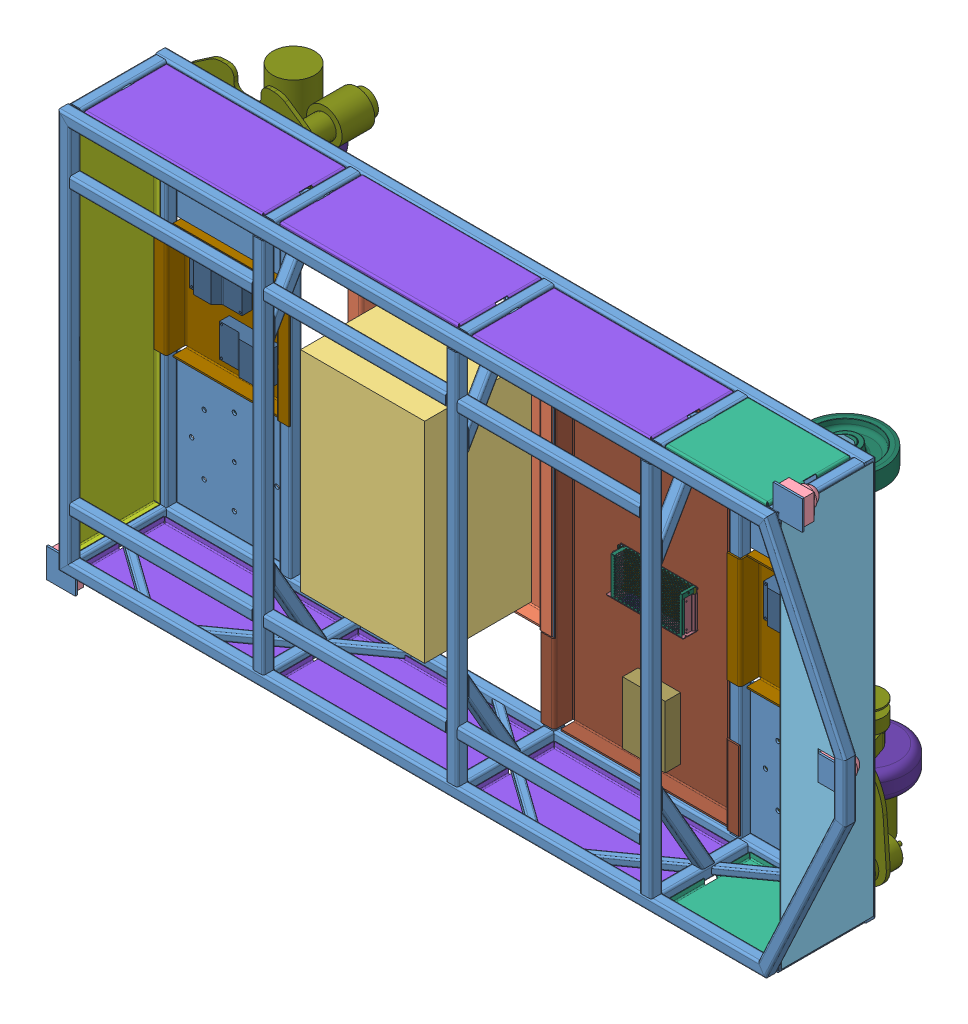
SolidWorks assembly spartaco_bot, configuration Default. Lengths in mm.
Overall size (2090 1155 574.19).
68 component instances, 36 part files, 77 mates.
Components (placement in the parent):
- 00-P-PT0151-1: 00-P-PT0151 [Default<A macchina>] at (-901.7891 -500.1516 -100.979) x (0 -1 0) z (-1 0 0) size (1155 285 2090)
- 00-P-PT0154-1: 00-P-PT0154 [Default] at (-151.7891 -0.1516 -135.979) x (1 0 0) z (0 -1 0) size (525 54 559)
- batteria-1: batteria [Default] at (-151.7891 -0.1516 -131.979) x (0 -1 0) z (-1 0 0) size (569 275 320)
- lidar-1: lidar [Default] at (940.7109 542.3484 129.021) x (0 -1 0) z (0 0 -1) size (73 65 60)
- lidar-2: lidar [Default] at (1050.7109 -0.1516 134.021) x (-1 0 0) z (0 0 -1) size (73 65 60)
- lidar-3: lidar [Default] at (-944.2891 -547.6516 129.021) x (0 1 0) z (0 0 -1) size (73 65 60)
- Parte13-1: Parte13 [Default] at (914.7109 -0.1516 -107.479) x (0 1 0) z (1 0 0) size (1015 241.5 195)
- Parte14-1: Parte14 [Default] at (750.7109 -515.1516 21.521) x (1 0 0) z (0 -1 0) size (265 215 15)
- Parte14-2: Parte14 [Default] at (745.7109 514.8484 21.521) x (-1 0 0) z (0 1 0) size (265 215 15)
- 00-P-PT0152-1: 00-P-PT0152 [Default] at (-916.7891 -2.6516 21.521) x (0 1 0) z (-1 0 0) size (965 215 15)
- 00-P-PT0153-1: 00-P-PT0153 [Default] at (-649.2891 514.8484 26.521) x (-1 0 0) z (0 1 0) size (465 215 15)
- 00-P-PT0153-2: 00-P-PT0153 [Default] at (-149.2891 514.8484 21.521) x (-1 0 0) z (0 1 0) size (465 215 15)
- 00-P-PT0153-3: 00-P-PT0153 [Default] at (350.7109 514.8484 26.521) x (-1 0 0) z (0 1 0) size (465 215 15)
- 00-P-PT0153-4: 00-P-PT0153 [Default] at (-654.2891 -515.1516 26.521) x (1 0 0) z (0 -1 0) size (465 215 15)
- 00-P-PT0153-5: 00-P-PT0153 [Default] at (-154.2891 -515.1516 26.521) x (1 0 0) z (0 -1 0) size (465 215 15)
- 00-P-PT0153-6: 00-P-PT0153 [Default] at (350.7109 -515.1516 26.521) x (1 0 0) z (0 -1 0) size (465 215 15)
- Parte17-1: Parte17 [Default] at (-1.7891 -0.1516 165.521) x (-1 0 0) z (0 1 0) size (2000 1.5 1000) (hidden)
- inverter_box-1: inverter_box [Default] at (738.2109 -0.1516 -120.7531) x (1 0 0) z (0 -1 0) size (350 54 299)
  - 00-P-PT0154-2-1: 00-P-PT0154-2 [Default] at (0 -15.2259 0) size (350 54 299)
  - minitraction_power_mockup-1: minitraction_power_mockup [Default] at (-36 -11.2259 -63) x (0 0 -1) z (0 1 0) size (85 130 40)
  - minitraction_power_mockup-2: minitraction_power_mockup [Default] at (36 -11.2259 63) x (0 0 1) z (0 1 0) size (85 130 40)
- inverter_box-2: inverter_box [Default] at (-741.7891 -0.1516 -120.7531) x (1 0 0) z (0 -1 0) size (350 54 299)
  - 00-P-PT0154-2-1: 00-P-PT0154-2 [Default] at (0 -15.2259 0) size (350 54 299)
  - minitraction_power_mockup-1: minitraction_power_mockup [Default] at (-36 -11.2259 -63) x (0 0 -1) z (0 1 0) size (85 130 40)
  - minitraction_power_mockup-2: minitraction_power_mockup [Default] at (36 -11.2259 63) x (0 0 1) z (0 1 0) size (85 130 40)
- electric_box-1: electric_box [Default] at (338.2109 -0.1516 -126.875) x (1 0 0) z (0 -1 0) size (510 54 969)
  - 00-P-PT0154-3-1: 00-P-PT0154-3 [Default] at (0 -9.104 0) size (510 54 969)
  - panda_mockup-1: panda_mockup [Default] at (0 -1.504 360.5) x (1 0 0) z (0 -1 0) size (110 160 39.6)
  - SD-100C-12-1: SD-100C-12 [Default] at (0 -3.604 71.625) size (199.09 37.75 98.27)
    - SD-100C-12.stp-1: SD-100C-12.stp [Default] at origin size (199.09 37.75 98.27)
      - SD-100-20201028.stp.stp-1: SD-100-20201028.stp.stp [Default] at origin size (199.09 37.75 98.27)
        - SD-100_STP.ASM.stp-1: SD-100_STP.ASM.stp [Default] at origin size (199.09 37.75 98.27)
          - SD-100_1_ASM.ASM.stp-1: SD-100_1_ASM.ASM.stp [Default] at origin size (199 37.75 98.27)
            - 902-D-80_ASM.ASM.stp-1: 902-D-80_ASM.ASM.stp [Default] at origin size (199 37.75 97.75)
              - 902-D-119_PRT.PRT.stp-1: 902-D-119_PRT.PRT.stp [Default] at origin size (199 37.75 97.75)
              - NUT_PRT.PRT.stp-1: NUT_PRT.PRT.stp [Default] at (-111.528 -1.5 -40.7894) x (-1 0 0) z (0 1 0) size (8 6.93 6)
            - 902-T_PRT.PRT.stp-1: 902-T_PRT.PRT.stp [Default] at (96.5 36.1 -49.375) x (-1 0 0) z (0 0 -1) size (195.5 36.02 96.52)
            - MYLAR_PRT.PRT.stp-1: MYLAR_PRT.PRT.stp [Default] at (79.2081 1.5 46.5396) x (-1 0 0) z (0 -1 0) size (197 95 0.5)
            - HS2_PRT.PRT.stp-1: HS2_PRT.PRT.stp [Default] at (-64.5 -80.2586 -88.3567) x (0 0 1) z (-1 0 0) size (6.4 28 55)
            - PCB_PRT.PRT.stp-1: PCB_PRT.PRT.stp [Default] at (-189.5595 4.5 45.0362) x (1 0 0) z (0 1 0) size (194 95 1.6)
          - T44-BS1R05370120201023_STP.ASM.stp-1: T44-BS1R05370120201023_STP.ASM.stp [Default] at (-82.3888 6.1 -32.875) x (0 0 1) z (0 1 0) size (69.8 18 18.8)
            - 6_PRT.PRT.stp-1: 6_PRT.PRT.stp [Default] at origin size (7.51 7.5 3.96)
            - 2_PRT.PRT.stp-1: 2_PRT.PRT.stp [Default] at origin size (7.5 7.5 3.96)
            - 3_PRT.PRT.stp-1: 3_PRT.PRT.stp [Default] at origin size (7.51 7.5 3.96)
            - 4_PRT.PRT.stp-1: 4_PRT.PRT.stp [Default] at (0 0.8 0) size (69.8 18 18.8)
            - 5_PRT.PRT.stp-1: 5_PRT.PRT.stp [Default] at origin size (7.51 7.5 3.96)
            - 6_PRT_1.PRT.stp-1: 6_PRT_1.PRT.stp [Default] at (9.5 0 0) size (7.51 7.5 3.96)
            - 6_PRT_1_1.PRT.stp-1: 6_PRT_1_1.PRT.stp [Default] at (19 0 0) size (7.51 7.5 3.96)
            - 6_PRT_1_1_1.PRT.stp-1: 6_PRT_1_1_1.PRT.stp [Default] at (28.5 0 0) size (7.51 7.5 3.96)
  - SD-25C-12-1: SD-25C-12 [Default] at (266.6665 2.696 -156.4754) x (1 0 0) z (0 1 0) size (99.05 97.03 36.06)
    - SD-25C-12.stp-1: SD-25C-12.stp [Default] at origin size (99.05 97.03 36.06)
      - RS-50_ASM_15.ASM.stp-1: RS-50_ASM_15.ASM.stp [Default] at origin size (99.05 97.03 36.06)
        - TN1_2.PRT.stp-1: TN1_2.PRT.stp [Default] at (-301.0065 335.8998 37.1723) x (0 0 -1) z (-1 0 0) size (15.25 49.25 14.66)
        - RS-50-CASE-T_21.PRT.stp-1: RS-50-CASE-T_21.PRT.stp [Default] at (0 1.5 1) size (97.05 96.6 36.06)
        - RS-50-CASE-D_28.PRT.stp-1: RS-50-CASE-D_28.PRT.stp [Default] at (-0.5 0.5 0) size (98.5 97 35)
        - RS-50-PCB_2.PRT.stp-1: RS-50-PCB_2.PRT.stp [Default] at (0 -0.6 -0.2033) size (98 95 1.6)
- piastra_pivot-1: piastra_pivot [Default] at (738.2109 324.8484 -120.979) x (1 0 0) z (0 0 -1) size (135 110 24.79)
- piastra_pivot-2: piastra_pivot [Default] at (-741.7891 -325.1516 -120.979) x (-1 0 0) z (0 0 -1) size (135 110 24.79)
- pivot-1: pivot [Default] at (680.4109 360.3484 -268.969) x (1 0 0) z (0 -1 0) size (183.58 152.49 93)
- wheel_200-1: wheel_200 [Default] at (680.4109 324.8484 -268.969) x (0 -1 0) z (0.453106 0 0.891457) size (62.5 200 200)
- pivot-2: pivot [Default] at (-799.5891 -289.6516 -268.969) x (1 0 0) z (0 -1 0) size (183.58 152.49 93)
- wheel_200-2: wheel_200 [Default] at (-799.5891 -325.1516 -268.969) x (0 -1 0) z (-0.745199 0 -0.666842) size (62.5 200 200)
- MRT05-1: MRT05 [Default] at (-725.5724 364.1588 -208.5704) x (1 0 0) z (0 -1 0) size (337.24 275.67 360.81)
  - MRT05-1: MRT05 [Default] at (-16.2167 -3.4086 117.2864) x (-1 0 0) z (0 0 -1) size (337.24 211.1 360.81)
  - MRT05_wheel-1: MRT05_wheel [Default] at (-16.2167 -60.4032 39.3104) x (0 0 1) z (-0.935001 -0.354644 0) size (71 198 198)
- MRT05-2: MRT05 [Default] at (721.9942 -364.4621 -208.5704) x (-1 0 0) z (0 1 0) size (337.24 275.67 360.81)
  - MRT05-1: MRT05 [Default] at (-16.2167 -3.4086 117.2864) x (-1 0 0) z (0 0 -1) size (337.24 211.1 360.81)
  - MRT05_wheel-1: MRT05_wheel [Default] at (-16.2167 -60.4032 39.3104) x (0 0 1) z (-0.935001 -0.354644 0) size (71 198 198)
Mates (geometry in assembly coordinates):
- Coincidente1: coordinate: unknown of 00-P-PT0151-1
- Coincidente2: coincident anti-aligned: plane of 00-P-PT0151-1 through (108.0109 -500.1516 -85.979) normal (0 0 1); plane of 00-P-PT0154-1 through (80.7109 -272.6516 -85.979) normal (0 0 -1)
- Larghezza1: width aligned: plane of 00-P-PT0151-1 through (-901.7891 484.8484 -91.179) normal (0 -1 0); plane of 00-P-PT0151-1 through (898.2109 -485.1516 -91.179) normal (0 1 0); plane of 00-P-PT0154-1 through (-151.7891 -279.6516 -135.979) normal (0 -1 0); plane of 00-P-PT0154-1 through (-151.7891 279.3484 -135.979) normal (0 1 0)
- Larghezza2: width anti-aligned: plane of 00-P-PT0151-1 through (83.2109 -500.1516 -110.779) normal (-1 0 0); plane of 00-P-PT0151-1 through (-386.7891 -500.1516 -91.179) normal (1 0 0); plane of 00-P-PT0154-1 through (80.7109 -272.6516 -135.979) normal (1 0 0); plane of 00-P-PT0154-1 through (-384.2891 -272.6516 -135.979) normal (-1 0 0)
- Coincidente4: coincident anti-aligned: plane of 00-P-PT0154-1 through (-384.2891 -272.6516 -131.979) normal (0 0 1); plane of batteria-1 through (-151.7891 -0.1516 -131.979) normal (0 0 -1)
- Larghezza3: width aligned: plane of 00-P-PT0154-1 through (-380.2891 -272.6516 -135.979) normal (1 0 0); plane of 00-P-PT0154-1 through (76.7109 -272.6516 -135.979) normal (-1 0 0); plane of batteria-1 through (8.2109 270.3484 143.021) normal (1 0 0); plane of batteria-1 through (-311.7891 270.3484 143.021) normal (-1 0 0)
- Larghezza4: width anti-aligned: plane of 00-P-PT0154-1 through (-151.7891 275.3484 -135.979) normal (0 -1 0); plane of 00-P-PT0154-1 through (-151.7891 -275.6516 -135.979) normal (0 1 0); plane of batteria-1 through (-311.7891 270.3484 143.021) normal (0 1 0); plane of batteria-1 through (-311.7891 -270.6516 143.021) normal (0 -1 0)
- Coincidente24: coincident anti-aligned: plane of 00-P-PT0151-1 through (-901.7891 -500.1516 129.021) normal (0 0 -1); plane of lidar-3 through (-944.2891 -547.6516 129.021) normal (0 0 1)
- Coincidente25: coincident anti-aligned: plane of 00-P-PT0151-1 through (-901.7891 -500.1516 134.0209) normal (0 0 -1); plane of lidar-2 through (1050.7109 -0.1516 134.021) normal (0 0 1)
- Coincidente26: coincident aligned: plane of 00-P-PT0151-1 through (-976.7891 -580.1516 129.021) normal (0 -1 0); plane of lidar-3 through (-911.7891 -580.1516 89.521) normal (0 -1 0)
- Coincidente27: coincident aligned: plane of 00-P-PT0151-1 through (-976.7891 -505.1516 129.021) normal (-1 0 0); plane of lidar-3 through (-976.7891 -580.1516 89.521) normal (-1 0 0)
- Coincidente28: coincident anti-aligned: plane of 00-P-PT0151-1 through (-901.7891 -500.1516 129.021) normal (0 0 -1); plane of lidar-1 through (940.7109 542.3484 129.021) normal (0 0 1)
- Coincidente29: coincident aligned: plane of 00-P-PT0151-1 through (973.2109 574.8484 129.021) normal (1 0 0); plane of lidar-1 through (973.2109 574.8484 89.521) normal (1 0 0)
- Coincidente30: coincident aligned: plane of 00-P-PT0151-1 through (898.2109 574.8484 129.021) normal (0 1 0); plane of lidar-1 through (908.2109 574.8484 89.521) normal (0 1 0)
- Larghezza15: width anti-aligned: plane of Parte13-1 through (1088.2109 -37.6516 134.022) normal (0 1 0); plane of Parte13-1 through (1088.2109 37.3484 134.022) normal (0 -1 0); plane of 00-P-PT0151-1 through (1083.2109 -32.6516 139.021) normal (0 -1 0); plane of 00-P-PT0151-1 through (1083.2109 32.3484 139.021) normal (0 1 0)
- Coincidente36: coincident anti-aligned: plane of 00-P-PT0151-1 through (883.2109 -490.3516 149.021) normal (-1 0 0); plane of Parte14-1 through (883.2109 -515.1516 21.521) normal (1 0 0)
- Coincidente37: coincident anti-aligned: plane of 00-P-PT0151-1 through (898.2109 -490.3516 -85.979) normal (0 0 1); plane of Parte14-1 through (750.7109 -515.1516 -85.979) normal (0 0 -1)
- Coincidente38: coincident aligned: plane of 00-P-PT0151-1 through (898.2109 -515.1516 -110.779) normal (0 -1 0); plane of Parte14-1 through (750.7109 -515.1516 21.521) normal (0 -1 0)
- Coincidente39: coincident aligned: plane of 00-P-PT0151-1 through (-901.7891 514.8484 -110.779) normal (0 1 0); plane of Parte14-2 through (745.7109 514.8484 21.521) normal (0 1 0)
- Coincidente40: coincident anti-aligned: plane of 00-P-PT0151-1 through (613.2109 490.0484 149.021) normal (1 0 0); plane of Parte14-2 through (613.2109 514.8484 21.521) normal (-1 0 0)
- Coincidente41: coincident anti-aligned: plane of 00-P-PT0151-1 through (-901.7891 490.0484 -85.979) normal (0 0 1); plane of Parte14-2 through (745.7109 514.8484 -85.979) normal (0 0 -1)
- Coincidente42: coincident aligned: plane of 00-P-PT0151-1 through (-901.7891 514.8484 -110.779) normal (0 1 0); plane of 00-P-PT0153-1 through (-649.2891 514.8484 26.521) normal (0 1 0)
- Coincidente43: coincident anti-aligned: plane of 00-P-PT0151-1 through (-416.7891 509.6484 149.021) normal (-1 0 0); plane of 00-P-PT0153-1 through (-416.7891 514.8484 26.521) normal (1 0 0)
- Coincidente44: coincident anti-aligned: plane of 00-P-PT0151-1 through (-901.7891 509.6484 134.021) normal (0 0 -1); plane of 00-P-PT0153-1 through (-649.2891 514.8484 134.021) normal (0 0 1)
- Coincidente45: coincident anti-aligned: plane of 00-P-PT0151-1 through (-891.9891 -500.1516 -85.979) normal (0 0 1); plane of 00-P-PT0152-1 through (-916.7891 -2.6516 -85.979) normal (0 0 -1)
- Coincidente46: coincident anti-aligned: plane of 00-P-PT0151-1 through (-911.5891 -485.1516 149.021) normal (0 1 0); plane of 00-P-PT0152-1 through (-916.7891 -485.1516 21.521) normal (0 -1 0)
- Coincidente47: coincident aligned: plane of 00-P-PT0151-1 through (-916.7891 -500.1516 139.221) normal (-1 0 0); plane of 00-P-PT0152-1 through (-916.7891 -2.6516 21.521) normal (-1 0 0)
- Coincidente48: coincident aligned: plane of 00-P-PT0151-1 through (-901.7891 514.8484 -110.779) normal (0 1 0); plane of 00-P-PT0153-3 through (350.7109 514.8484 26.521) normal (0 1 0)
- Coincidente49: coincident anti-aligned: plane of 00-P-PT0151-1 through (-901.7891 509.6484 134.021) normal (0 0 -1); plane of 00-P-PT0153-3 through (350.7109 514.8484 134.021) normal (0 0 1)
- Coincidente50: coincident anti-aligned: plane of 00-P-PT0151-1 through (583.2109 509.6484 149.021) normal (-1 0 0); plane of 00-P-PT0153-3 through (583.2109 514.8484 26.521) normal (1 0 0)
- Coincidente51: coincident anti-aligned: plane of 00-P-PT0151-1 through (-901.7891 490.0484 -85.979) normal (0 0 1); plane of 00-P-PT0153-2 through (-149.2891 514.8484 -85.979) normal (0 0 -1)
- Coincidente52: coincident aligned: plane of 00-P-PT0151-1 through (-901.7891 514.8484 -110.779) normal (0 1 0); plane of 00-P-PT0153-2 through (-149.2891 514.8484 21.521) normal (0 1 0)
- Coincidente53: coincident anti-aligned: plane of 00-P-PT0151-1 through (83.2109 509.6484 149.021) normal (-1 0 0); plane of 00-P-PT0153-2 through (83.2109 514.8484 21.521) normal (1 0 0)
- Coincidente54: coincident aligned: plane of 00-P-PT0151-1 through (898.2109 -515.1516 -110.779) normal (0 -1 0); plane of 00-P-PT0153-4 through (-654.2891 -515.1516 26.521) normal (0 -1 0)
- Coincidente55: coincident anti-aligned: plane of 00-P-PT0151-1 through (-886.7891 -509.9516 149.021) normal (1 0 0); plane of 00-P-PT0153-4 through (-886.7891 -515.1516 26.521) normal (-1 0 0)
- Coincidente56: coincident anti-aligned: plane of 00-P-PT0151-1 through (898.2109 -509.9516 134.021) normal (0 0 -1); plane of 00-P-PT0153-4 through (-654.2891 -515.1516 134.021) normal (0 0 1)
- Coincidente57: coincident aligned: plane of 00-P-PT0151-1 through (898.2109 -515.1516 -110.779) normal (0 -1 0); plane of 00-P-PT0153-5 through (-154.2891 -515.1516 26.521) normal (0 -1 0)
- Coincidente58: coincident anti-aligned: plane of 00-P-PT0151-1 through (898.2109 -509.9516 134.021) normal (0 0 -1); plane of 00-P-PT0153-5 through (-154.2891 -515.1516 134.021) normal (0 0 1)
- Coincidente59: coincident anti-aligned: plane of 00-P-PT0151-1 through (-386.7891 -509.9516 149.021) normal (1 0 0); plane of 00-P-PT0153-5 through (-386.7891 -515.1516 26.521) normal (-1 0 0)
- Coincidente60: coincident aligned: plane of 00-P-PT0151-1 through (898.2109 -515.1516 -110.779) normal (0 -1 0); plane of 00-P-PT0153-6 through (350.7109 -515.1516 26.521) normal (0 -1 0)
- Coincidente61: coincident anti-aligned: plane of 00-P-PT0151-1 through (898.2109 -509.9516 134.021) normal (0 0 -1); plane of 00-P-PT0153-6 through (350.7109 -515.1516 134.021) normal (0 0 1)
- Coincidente62: coincident anti-aligned: plane of 00-P-PT0151-1 through (583.2109 -490.3516 149.021) normal (-1 0 0); plane of 00-P-PT0153-6 through (583.2109 -515.1516 26.521) normal (1 0 0)
- Larghezza16: width aligned: plane of 00-P-PT0151-1 through (898.2109 -515.1516 139.221) normal (0 -1 0); plane of 00-P-PT0151-1 through (-901.7891 514.8484 139.221) normal (0 1 0); plane of Parte17-1 through (898.2109 -500.1516 164.021) normal (0 -1 0); plane of Parte17-1 through (898.2109 499.8484 164.021) normal (0 1 0)
- Coincidente64: coincident anti-aligned: plane of 00-P-PT0151-1 through (608.0109 -500.1516 164.021) normal (0 0 1); plane of Parte17-1 through (-1.7891 -0.1516 164.021) normal (0 0 -1)
- Coincidente66: coincident aligned: plane of 00-P-PT0151-1 through (1083.2109 32.3484 139.021) normal (1 0 0); plane of lidar-2 through (1083.2109 32.3484 94.521) normal (1 0 0)
- Coincidente67: coincident aligned: plane of 00-P-PT0151-1 through (1083.2109 -32.6516 139.021) normal (0 -1 0); plane of lidar-2 through (1083.2109 -32.6516 94.521) normal (0 -1 0)
- Coincidente69: coincident: line of 00-P-PT0151-1 through (1098.2109 70.947 149.021) axis (0 -1 0); plane of Parte17-1 through (1098.2109 -74.1516 164.021) normal (1 0 0)
- Larghezza20: width anti-aligned: plane of Parte13-1 through (1013.2109 37.3484 134.022) normal (1 0 0); plane of 00-P-PT0151-1 through (1088.2109 37.3484 134.022) normal (-1 0 0); plane of Parte13-1 through (1018.2109 32.3484 139.021) normal (-1 0 0); plane of 00-P-PT0151-1 through (1083.2109 32.3484 139.021) normal (1 0 0)
- Coincidente76: coincident anti-aligned: plane of 00-P-PT0151-1 through (1108.0109 70.947 134.021) normal (0 0 -1); plane of Parte13-1 through (914.7109 507.3484 134.021) normal (0 0 1)
- Larghezza21: width anti-aligned: plane of 00-P-PT0151-1 through (883.2109 499.8484 -91.179) normal (-1 0 0); plane of inverter_box-1/00-P-PT0154-2-1 through (593.2109 -500.1516 -91.179) normal (1 0 0); plane of 00-P-PT0151-1 through (883.2109 -142.6516 -135.979) normal (1 0 0); plane of inverter_box-1/00-P-PT0154-2-1 through (593.2109 -142.6516 -135.979) normal (-1 0 0)
- Coincidente78: coincident anti-aligned: plane of 00-P-PT0151-1 through (588.0109 -500.1516 -85.979) normal (0 0 1); plane of inverter_box-1/00-P-PT0154-2-1 through (593.2109 -142.6516 -85.979) normal (0 0 -1)
- Larghezza22: width aligned: plane of 00-P-PT0151-1 through (898.2109 149.8484 -120.979) normal (0 -1 0); plane of inverter_box-1/00-P-PT0154-2-1 through (898.2109 -150.1516 -120.979) normal (0 1 0); plane of 00-P-PT0151-1 through (738.2109 -149.6516 -135.979) normal (0 -1 0); plane of inverter_box-1/00-P-PT0154-2-1 through (738.2109 149.3484 -135.979) normal (0 1 0)
- Larghezza23: width aligned: plane of 00-P-PT0151-1 through (-581.7891 -150.1516 -120.979) normal (0 1 0); plane of inverter_box-2/00-P-PT0154-2-1 through (-581.7891 149.8484 -120.979) normal (0 -1 0); plane of 00-P-PT0151-1 through (-741.7891 149.3484 -135.979) normal (0 1 0); plane of inverter_box-2/00-P-PT0154-2-1 through (-741.7891 -149.6516 -135.979) normal (0 -1 0)
- Coincidente79: coincident anti-aligned: plane of 00-P-PT0151-1 through (-571.9891 -500.1516 -85.979) normal (0 0 1); plane of inverter_box-2/00-P-PT0154-2-1 through (-596.7891 -142.6516 -85.979) normal (0 0 -1)
- Larghezza24: width aligned: plane of 00-P-PT0151-1 through (-886.7891 -500.1516 -91.179) normal (1 0 0); plane of inverter_box-2/00-P-PT0154-2-1 through (-596.7891 -500.1516 -110.779) normal (-1 0 0); plane of 00-P-PT0151-1 through (-596.7891 -142.6516 -135.979) normal (1 0 0); plane of inverter_box-2/00-P-PT0154-2-1 through (-886.7891 -142.6516 -135.979) normal (-1 0 0)
- Coincidente80: coincident anti-aligned: plane of 00-P-PT0151-1 through (588.0109 -500.1516 -85.979) normal (0 0 1); plane of electric_box-1/00-P-PT0154-3-1 through (563.2109 -477.6516 -85.979) normal (0 0 -1)
- Larghezza25: width aligned: plane of 00-P-PT0151-1 through (898.2109 -485.1516 -91.179) normal (0 1 0); plane of electric_box-1/00-P-PT0154-3-1 through (-901.7891 484.8484 -91.179) normal (0 -1 0); plane of 00-P-PT0151-1 through (338.2109 484.3484 -135.979) normal (0 1 0); plane of electric_box-1/00-P-PT0154-3-1 through (338.2109 -484.6516 -135.979) normal (0 -1 0)
- Larghezza26: width aligned: plane of 00-P-PT0151-1 through (113.2109 -500.1516 -91.179) normal (1 0 0); plane of electric_box-1/00-P-PT0154-3-1 through (563.2109 -500.1516 -110.779) normal (-1 0 0); plane of 00-P-PT0151-1 through (563.2109 -477.6516 -135.979) normal (1 0 0); plane of electric_box-1/00-P-PT0154-3-1 through (113.2109 -477.6516 -135.979) normal (-1 0 0)
- Coincidente83: coincident anti-aligned: line of 00-P-PT0151-1 through (738.2109 324.8484 -120.979) axis (0 0 1); line of piastra_pivot-1 through (738.2109 324.8484 -124.979) axis (0 0 -1)
- Coincidente84: coincident anti-aligned: plane of 00-P-PT0151-1 through (-901.7891 -500.1516 -120.979) normal (0 0 -1); plane of piastra_pivot-1 through (738.2109 324.8484 -120.979) normal (0 0 1)
- Parallelo6: parallel aligned: plane of 00-P-PT0151-1 through (898.2109 499.8484 -120.979) normal (0 1 0); plane of piastra_pivot-1 through (670.7109 379.8484 -123.979) normal (0 1 0)
- Coincidente86: coincident anti-aligned: line of 00-P-PT0151-1 through (-741.7891 -325.1516 -120.979) axis (0 0 1); line of piastra_pivot-2 through (-741.7891 -325.1516 -124.979) axis (0 0 -1)
- Coincidente87: coincident anti-aligned: plane of 00-P-PT0151-1 through (-2381.7891 -1150.1516 -120.979) normal (0 0 -1); plane of piastra_pivot-2 through (-741.7891 -325.1516 -120.979) normal (0 0 1)
- Parallelo7: parallel aligned: plane of 00-P-PT0151-1 through (-581.7891 -500.1516 -120.979) normal (0 -1 0); plane of piastra_pivot-2 through (-674.2891 -380.1516 -123.979) normal (0 -1 0)
- Coincidente88: coincident anti-aligned: line of piastra_pivot-1 through (738.2109 324.8484 -124.979) axis (0 0 -1); line of pivot-1 through (738.2109 324.8484 -262.7486) axis (0 0 1)
- Coincidente89: coincident anti-aligned: plane of piastra_pivot-1 through (774.7109 324.8484 -124.979) normal (0 0 -1); plane of pivot-1 through (738.2109 324.8484 -124.979) normal (0 0 1)
- Coincidente93: coincident anti-aligned: line of pivot-2 through (-799.5891 -357.6516 -268.969) axis (0 1 0); line of wheel_200-2 through (-799.5891 -170.4115 -268.969) axis (0 -1 0)
- Coincidente94: coincident anti-aligned: line of piastra_pivot-2 through (-741.7891 -325.1516 -124.979) axis (0 0 -1); line of pivot-2 through (-741.7891 -325.1516 -262.7486) axis (0 0 1)
- Coincidente95: coincident anti-aligned: plane of piastra_pivot-2 through (-778.2891 -325.1516 -124.979) normal (0 0 -1); plane of pivot-2 through (-741.7891 -325.1516 -124.979) normal (0 0 1)
- Coincidente100: coincident anti-aligned: line of pivot-2 through (-799.5891 -357.6516 -268.969) axis (0 1 0); line of wheel_200-2 through (-799.5891 -170.4115 -268.969) axis (0 -1 0)
- Coincidente102: coincident: point of pivot-2; point of wheel_200-2
- Coincidente104: coincident: point of pivot-1; point of wheel_200-1
- Coincidente105: coincident anti-aligned: line of pivot-1 through (680.4109 292.3484 -268.969) axis (0 1 0); line of wheel_200-1 through (680.4109 479.5885 -268.969) axis (0 -1 0)
- Coincidente106: coincident anti-aligned: line of 00-P-PT0151-1 through (738.2109 -325.1516 -120.979) axis (0 0 1); line of MRT05-2/MRT05-1 through (738.2109 -325.1516 -75.7493) axis (0 0 -1)
- Coincidente107: coincident anti-aligned: plane of 00-P-PT0151-1 through (-901.7891 -1150.1516 -120.979) normal (0 0 -1); plane of MRT05-2/MRT05-1 through (738.2109 -200.6516 -120.979) normal (0 0 1)
- Coincidente108: coincident anti-aligned: line of 00-P-PT0151-1 through (-741.7891 324.8484 -120.979) axis (0 0 1); line of MRT05-1/MRT05-1 through (-741.7891 324.8484 -75.7493) axis (0 0 -1)
- Coincidente109: coincident anti-aligned: plane of 00-P-PT0151-1 through (-2381.7891 -500.1516 -120.979) normal (0 0 -1); plane of MRT05-1/MRT05-1 through (-741.7891 200.3484 -120.979) normal (0 0 1)
